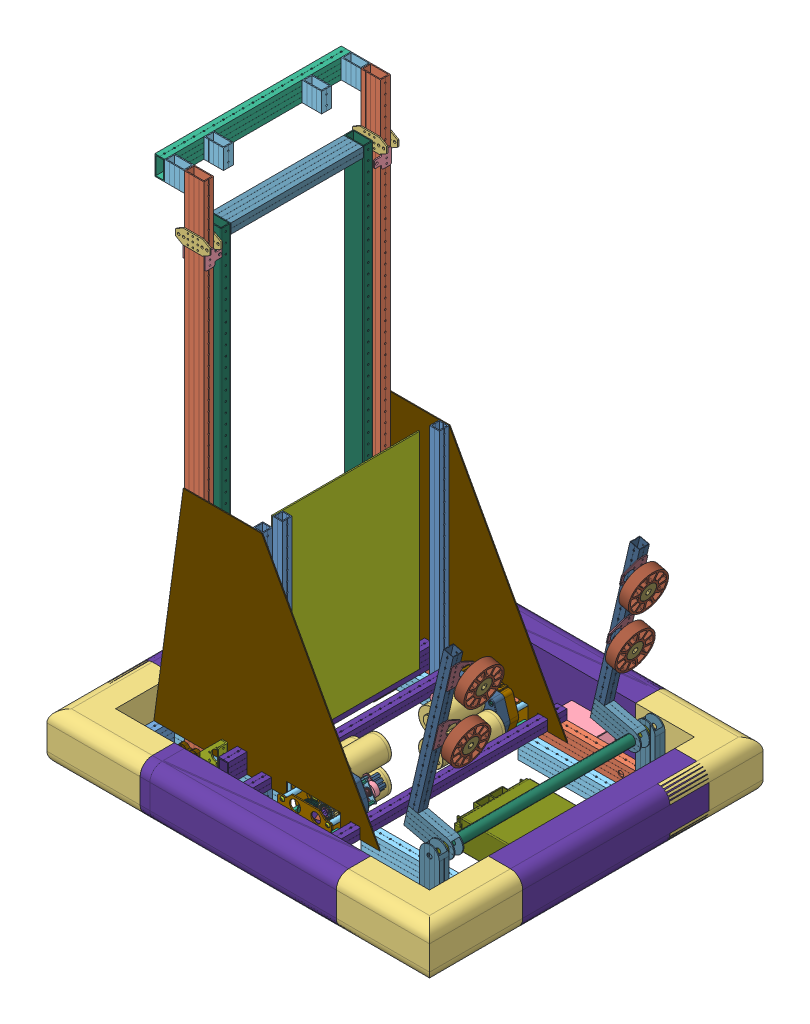
SolidWorks assembly FINAL BOT, configuration Default. Lengths in mm.
Overall size (1308.1 2133.6 883.55).
451 component instances, 126 part files, 82 mates.
Components (placement in the parent):
- Test Base 3-1: Test Base 3 [Default] at (-213.2986 -131.6714 217.4582) size (990.6 641.86 863.6)
  - Base Rear Rail-1: Base Rear Rail [Default] at (282.1219 360.9185 104.1623) size (25.4 50.8 685.8)
  - Base Side Rail-1: Base Side Rail [Default] at (1044.1219 360.9185 789.9623) x (0 0 1) z (-1 0 0) size (25.4 50.8 762)
  - Base Side Rail-2: Base Side Rail [Default] at (1044.1219 360.9185 231.1623) x (0 0 1) z (-1 0 0) size (25.4 50.8 762)
  - Blue Bumper-1: Blue Bumper [Default] at (1171.1219 335.5185 942.3623) x (0 0 -1) z (1 0 0) size (241.3 127 241.3)
  - Blue Bumper-2: Blue Bumper [Default] at (1171.1219 335.5185 78.7623) x (-1 0 0) z (0 0 -1) size (241.3 127 241.3)
  - Bumper Support Bar-2: Bumper Support Bar [Default] at (879.0219 335.5185 166.0294) x (0 0 1) z (-1 0 0) size (50.8 50.8 114.3)
  - Bumper Support Bar-4: Bumper Support Bar [Default] at (586.9219 335.5185 166.0294) x (0 0 1) z (-1 0 0) size (50.8 50.8 114.3)
  - Bumper Support Bar-7: Bumper Support Bar [Default] at (586.9219 335.5185 801.0294) x (0 0 1) z (-1 0 0) size (50.8 50.8 114.3)
  - Bumper Support Bar-8: Bumper Support Bar [Default] at (879.0219 335.5185 801.0294) x (0 0 1) z (-1 0 0) size (50.8 50.8 114.3)
  - Base Side Rail Internal-1: Base Side Rail Internal [Default] at (-175.0781 360.9185 713.7623) x (0 0 -1) z (1 0 0) size (25.4 50.8 279.4)
  - Base Side Rail Internal-4: Base Side Rail Internal [Default] at (1044.1219 360.9185 307.3623) x (0 0 1) z (-1 0 0) size (25.4 50.8 279.4)
  - Base Front Rail-1: Base Front Rail [Default] at (1069.5219 360.9185 104.1623) size (25.4 50.8 152.4)
  - 3 CIM Ball Shifter with WCD Output-1: 3 CIM Ball Shifter with WCD Output [Default] at (711.3612 400.7203 682.3171) x (0 1 0) z (0 0 1) size (169.11 183.68 312.65)
    - 217-2733-001 Rev2-1: 217-2733-001 Rev2 [Default] at (0 53.4162 37.6682) x (0 0 1) z (-0.00054 -1 0) size (7.11 24.61 24.61)
    - 217-2733-001 Rev2-2: 217-2733-001 Rev2 [Default] at (0 53.4162 7.9248) x (0 0 -1) z (-0.038475 0.99926 0) size (7.11 24.61 24.61)
    - 217-2731-001 Rev2-1: 217-2731-001 Rev2 [Default] at (0 0 0.0381) x (-0.099212 0.995066 0) z (0.995066 0.099212 0) size (31.12 7.94 31.12)
    - 217-2789-001 Rev2-1: 217-2789-001 Rev2 [Default] at (0 0 43.2943) x (0 0 -1) z (-0.58471 0.811243 0) size (11.1 38.4 38.4)
    - 217-2778-001 Rev2_NCQ8A075-050M_1-1: 217-2778-001 Rev2_NCQ8A075-050M_1 [Default] at (0 0 -53.848) x (-0.707107 0.707107 0) z (0 0 1) size (31.75 33.34 39.88)
      - 217-2778-002_075A-1: 217-2778-002_075A [Default] at origin size (31.75 33.34 26.92)
      - 217-2778-003_075M-1: 217-2778-003_075M [Default] at (0 0 -8.85) x (0.866025 -0.5 0) z (0 0 1) size (18.95 18.95 35.27)
      - 217-2778-004_075-1: 217-2778-004_075 [Default] at (0 0 10.362) size (21 20.74 0.97)
    - 217-2428-012 Rev2-1: 217-2428-012 Rev2 [Default] at (0 0 -40.386) size (63.5 22.23 2.29)
    - 217-2428-005 Rev1-1: 217-2428-005 Rev1 [Default] at (25.4 0 -19.05) x (-0.557362 -0.83027 0) z (-0.83027 0.557362 0) size (7.33 38.98 6.35)
    - 217-2428-005 Rev1-2: 217-2428-005 Rev1 [Default] at (-25.4 0 -19.05) x (0.667436 0.744667 0) z (0.744667 -0.667436 0) size (7.33 38.98 6.35)
    - SCREW-832-0375-1: SCREW-832-0375 [Default] at (25.4 0 -42.5958) x (0 0 1) z (-0.875404 0.483392 0) size (11.73 7.92 7.92)
    - SCREW-832-0375-2: SCREW-832-0375 [Default] at (-25.4 0 -42.5958) x (0 0 1) z (-0.966319 0.257347 0) size (11.73 7.92 7.92)
    - SCREW-832-0375-3: SCREW-832-0375 [Default] at (25.4 0 5.3848) x (0 0 -1) z (1 0 0) size (11.73 7.92 7.92)
    - SCREW-832-0375-4: SCREW-832-0375 [Default] at (-25.4 0 5.3848) x (0 0 -1) z (0.941463 -0.337115 0) size (11.73 7.92 7.92)
    - SBS1_SBS-0632-0250-1: SBS1_SBS-0632-0250 [Default] at (15.494 0 -36.2458) x (0 0 -1) z (0.854303 -0.519775 0) size (8.57 6.68 6.65)
    - SBS1_SBS-0632-0250-2: SBS1_SBS-0632-0250 [Default] at (-15.494 0 -36.2458) x (0 0 -1) z (0.854303 -0.519775 0) size (8.57 6.68 6.65)
    - 217-4098-100 Rev1-1: 217-4098-100 Rev1 [Default] at (0 0 -16.927) x (-0.503316 0.864103 0) z (0 0 1) size (18.03 19.79 22.46)
      - 217-4098-006 Rev2-1: 217-4098-006 Rev2 [Default] at (0 0 -4.6312) x (0 -1 0) z (0 0 -1) size (18.09 11.02 22.46)
      - 217-4098-006 Rev2-2: 217-4098-006 Rev2 [Default] at (0 0 -4.6312) x (0 1 0) z (0 0 -1) size (18.09 11.02 22.46)
      - 217-3489-001 Rev1-1: 217-3489-001 Rev1 [Default] at (0 0 -4.6312) x (0 0 1) z (-0.980217 -0.197926 0) size (4.77 12.7 12.7)
      - 97633A130_97633A130_grv-1: 97633A130_97633A130_grv [Default] at (0 0 -7.33) x (0 0 -1) z (0.979861 0.199683 0) size (0.64 8.74 7.34)
      - 91251A107_91251A107-1: 91251A107_91251A107 [Default] at (-4.8375 -6.735 -9.4343) x (0 0.863883 -0.503692) z (-1 0 0) size (4.65 4.65 10.79)
      - 91251A107_91251A107-2: 91251A107_91251A107 [Default] at (4.8375 6.735 -9.4343) x (0 0.470889 -0.882193) z (1 0 0) size (4.65 4.65 10.79)
    - 217-2428-017 Rev2-1: 217-2428-017 Rev2 [Default] at (12.7 -21.997 -3.614) x (-0.578458 -0.815712 0) z (0 0 -1) size (14.73 14.73 7.37)
    - 217-2428-016 Rev3_Spur01-1: 217-2428-016 Rev3_Spur01 [Default] at (0 0 -3.614) x (0.873157 -0.48744 0) z (0 0 1) size (40.67 40.74 13.32)
    - 217-2428-019 Rev1-1: 217-2428-019 Rev1 [Default] at (12.7 -21.997 -20.6248) x (0.866025 0.5 0) z (0 0 1) size (50.8 19.05 1.57)
    - 217-2428-006 Rev1-1: 217-2428-006 Rev1 [Default] at (32.079 -14.2875 -9.525) x (-0.752416 0.658689 0) z (0.658689 0.752416 0) size (7.33 19.93 6.35)
    - 217-2428-006 Rev1-2: 217-2428-006 Rev1 [Default] at (-3.6662 -34.925 -9.525) x (0.84498 0.534798 0) z (0.534798 -0.84498 0) size (7.33 19.93 6.35)
    - SCREW-832-0375-5: SCREW-832-0375 [Default] at (32.079 -14.2875 4.7498) x (0 0 -1) z (0.980613 0.195955 0) size (11.73 7.92 7.92)
    - SCREW-832-0375-6: SCREW-832-0375 [Default] at (-3.6662 -34.925 5.3848) x (0 0 -1) z (-0.672515 -0.740083 0) size (11.73 7.92 7.92)
    - SCREW-832-0375-7: SCREW-832-0375 [Default] at (-3.6662 -34.925 -22.8346) x (0 0 1) z (0.948865 0.315681 0) size (11.73 7.92 7.92)
    - SCREW-832-0375-8: SCREW-832-0375 [Default] at (32.079 -14.2875 -22.8346) x (0 0 1) z (-0.875404 0.483392 0) size (11.73 7.92 7.92)
    - 217-2614-001_12t-1: 217-2614-001_12t [Default] at (36.9798 39.6868 15.8623) x (-0.087156 0.996195 0) z (0 0 1) size (18.29 18.29 19)
    - 217-2761-001 rev1-1: 217-2761-001 rev1 [Default] at (33.1943 39.3556 16.1) x (0.087156 -0.996195 0) z (0 0 1) size (2 2 20)
    - 217-2761-001 rev1-2: 217-2761-001 rev1 [Default] at (-40.7653 40.018 16.1) x (0.087156 0.996195 0) z (0 0 1) size (2 2 20)
    - 217-2614-001_12t-2: 217-2614-001_12t [Default] at (-36.9798 39.6868 15.8623) x (0.087156 0.996195 0) z (0 0 1) size (18.29 18.29 19)
    - 217-2614-001_12t-3: 217-2614-001_12t [Default] at (0 92.8624 15.8623) x (0.97459 0.223996 0) z (0 0 1) size (18.29 18.29 19)
    - 217-2761-001 rev1-3: 217-2761-001 rev1 [Default] at (-0.8512 96.5658 16.1) x (0.97459 0.223996 0) z (0 0 1) size (2 2 20)
    - 217-3195-002 rev2-1: 217-3195-002 rev2 [Default] at (0 0 50.546) x (-1 0 0) z (0 0 -1) size (114.31 152.24 24.96)
    - 217-3195-001 Rev1-1: 217-3195-001 Rev1 [Default] at origin size (113.41 152.24 26.86)
    - Nylock Nut_NNY2520-ZC-1: Nylock Nut_NNY2520-ZC [Default] at (48.8823 73.025 37.846) x (0 0.866025 -0.5) z (-1 0 0) size (12.85 11.89 7.62)
    - Nylock Nut_NNY2520-ZC-2: Nylock Nut_NNY2520-ZC [Default] at (48.8823 -3.175 37.846) x (0 0 -1) z (-1 0 0) size (12.85 11.89 7.62)
    - Nylock Nut_NNY2520-ZC-3: Nylock Nut_NNY2520-ZC [Default] at (44.45 85.725 7.8613) x (0 1 0) z (0 0 -1) size (12.85 11.89 7.62)
    - 276-1027-001-1: 276-1027-001 [Default] at (47.625 58.1787 6.35) x (0 1 0) z (-1 0 0) size (8.61 5.64 9.94)
    - 276-1027-001-2: 276-1027-001 [Default] at (-47.625 58.1787 6.35) x (0 -1 0) z (1 0 0) size (8.61 5.64 9.94)
    - SCREW-832-1750-1: SCREW-832-1750 [Default] at (-47.625 58.1787 47.0408) x (0 0 -1) z (-0.960822 -0.277167 0) size (46.66 7.92 7.92)
    - SCREW-832-1750-2: SCREW-832-1750 [Default] at (47.625 58.1787 47.0408) x (0 0 -1) z (-0.960822 -0.277167 0) size (46.66 7.92 7.92)
    - Nylock Nut_NNY2520-ZC-4: Nylock Nut_NNY2520-ZC [Default] at (44.45 -15.875 7.8613) x (0 1 0) z (0 0 -1) size (12.85 11.89 7.62)
    - 217-2428-004 Rev3-1: 217-2428-004 Rev3 [Default] at (0 53.4162 22.7711) x (-0.709585 0.70462 0) z (0 0 1) size (11 9.53 43.92)
    - SBS1_SBS-2520-1625SS-1: SBS1_SBS-2520-1625SS [Default] at (44.45 85.725 42.4688) x (0 0 -1) z (-0.251219 0.96793 0) size (45.3 11.2 11.18)
    - SBS1_SBS-2520-1625SS-2: SBS1_SBS-2520-1625SS [Default] at (44.45 -15.875 42.4688) x (0 0 -1) z (-0.251219 0.96793 0) size (45.3 11.2 11.18)
    - SBS1_SBS2520-1750-1: SBS1_SBS2520-1750 [Default] at (-44.45 85.725 7.4422) x (0 0 1) z (-0.031478 0.999504 0) size (48.48 11.22 11.17)
    - SBS1_SBS2520-1750-2: SBS1_SBS2520-1750 [Default] at (-44.45 -15.875 7.4422) x (0 0 1) z (-0.937114 -0.349025 0) size (48.48 11.22 11.17)
    - 217-2428-021 Rev1-1: 217-2428-021 Rev1 [Default] at (0 53.4162 9.5123) x (0.451333 -0.892356 0) z (0 0 1) size (15.88 15.88 3.17)
    - 217-2428-029 Rev1-1: 217-2428-029 Rev1 [Default] at (0 53.4162 36.957) x (0.999846 0.017557 0) z (0 0 1) size (15.88 15.88 1.12)
    - Grayhill Lock Washer-1: Grayhill Lock Washer [Default] at (12.7 -21.997 -18.6817) x (0.467173 -0.884166 0) z (0 0 1) size (19.69 19.69 0.74)
    - Grayhill Nut-1: Grayhill Nut [Default] at (12.7 -21.997 -17.0434) x (0.984088 0.177684 0) z (0 0 1) size (18.33 15.88 2.54)
    - 217-2000-1: 217-2000 [Default] at (0 92.8624 0) x (0 0 -1) z (0.223996 -0.97459 0) size (150.2 64.01 64.01)
    - 217-2000-2: 217-2000 [Default] at (-36.9798 39.6868 0) x (0 0 -1) z (0.996195 -0.087156 0) size (150.2 64.01 64.01)
    - 217-2000-3: 217-2000 [Default] at (36.9798 39.6868 0) x (0 0 -1) z (0.996195 0.087156 0) size (150.2 64.01 64.01)
    - Grahill Encoder-1: Grahill Encoder [Default] at (12.7 -21.997 -16.1798) x (-0.580071 0.814566 0) z (-0.814566 -0.580071 0) size (31.75 31.12 31.75)
    - 217-3195-009 Rev1_wcd 2-1: 217-3195-009 Rev1_wcd 2 [Default] at (0 85.725 50.546) x (-0.998427 -0.056065 0) z (0 0 1) size (12.7 12.7 41.27)
    - 217-3195-006 Rev1_WCD-1: 217-3195-006 Rev1_WCD [Default] at (-44.45 85.725 44.1452) x (0.5 0.866025 0) z (0 0 1) size (12.7 14.66 47.62)
    - 217-3195-009 Rev1_wcd 2-2: 217-3195-009 Rev1_wcd 2 [Default] at (0 -31.75 50.546) x (0.947633 0.319361 0) z (0 0 1) size (12.7 12.7 41.27)
    - 217-3195-006 Rev1_WCD-2: 217-3195-006 Rev1_WCD [Default] at (-44.45 -15.875 44.1452) x (0.5 -0.866025 0) z (0 0 1) size (12.7 14.66 47.62)
    - Nylock Nut_NNY2520-ZC-5: Nylock Nut_NNY2520-ZC [Default] at (0 -31.75 45.0723) x (-0.5 0.866025 0) z (0 0 -1) size (12.85 11.89 7.62)
    - Nylock Nut_NNY2520-ZC-6: Nylock Nut_NNY2520-ZC [Default] at (0 85.725 45.0723) x (-0.5 0.866025 0) z (0 0 -1) size (12.85 11.89 7.62)
    - SBS1_SBS-2520-2250-1: SBS1_SBS-2520-2250 [Default] at (0 -31.75 98.298) x (0 0 -1) z (-0.933488 -0.358607 0) size (61.18 11.22 11.17)
    - SBS1_SBS2520-0625ZC-1: SBS1_SBS2520-0625ZC [Default] at (-44.45 85.725 98.298) x (0 0 -1) z (0.400817 0.916158 0) size (19.57 11.22 11.17)
    - SBS1_SBS2520-0625ZC-2: SBS1_SBS2520-0625ZC [Default] at (-44.45 -15.875 98.298) x (0 0 -1) z (-0.75178 -0.659414 0) size (19.57 11.22 11.17)
    - SBS1_SBS-2520-2250-2: SBS1_SBS-2520-2250 [Default] at (0 85.725 98.298) x (0 0 -1) z (0.056677 -0.998393 0) size (61.18 11.22 11.17)
    - 217-3195-003 rev2-1: 217-3195-003 rev2 [Default] at (0 0 94.9452) size (88.62 139.7 3.17)
    - 217-2617-003 Rev1-1: 217-2617-003 Rev1 [Default] at (-39.878 35.5392 121.8535) x (-0.5 -0.866025 0) z (0 0 1) size (14.66 12.7 152.4)
    - 217-3109-001 Rev1-1: 217-3109-001 Rev1 [Default] at (-39.878 35.5392 49.1808) x (0 0 1) z (0.312889 -0.94979 0) size (7.94 28.57 28.57)
    - 217-2734-001 Rev3-1: 217-2734-001 Rev3 [Default] at (-39.878 35.5392 98.1202) x (1 0 0) z (0 1 0) size (31.12 7.94 31.12)
    - 217-2617-004 Rev1_97431A340_grv-1: 217-2617-004 Rev1_97431A340_grv [Default] at (-39.878 35.5392 54.8961) x (0 0 1) z (-0.124043 -0.992277 0) size (1.07 20.42 18.58)
    - 217-2617-004 Rev1_97431A340_grv-2: 217-2617-004 Rev1_97431A340_grv [Default] at (0 0 69.215) x (0 0 1) z (-0.124043 -0.992277 0) size (1.07 20.42 18.58)
    - 217-2702-001_20t-1: 217-2702-001_20t [Default] at (0 0 62.357) x (0.998435 0.055929 0) z (0 0 1) size (28.2 28.2 12.65)
    - 217-2715-002 Rev1_64t-1: 217-2715-002 Rev1_64t [Default] at (-39.878 35.5392 61.7541) x (0.866025 -0.5 0) z (0 0 1) size (84.3 84.3 12.65)
    - 217-2704-001_24-1: 217-2704-001_24 [Default] at (0 0 62.357) x (0.450781 0.892635 0) z (0 0 -1) size (33.29 33.29 12.65)
    - 217-2714-002 Rev1_60t-1: 217-2714-002 Rev1_60t [Default] at (-39.878 35.5392 61.7541) x (0.866025 -0.5 0) z (0 0 1) size (78.95 78.95 12.65)
    - 217-3221-002 Rev1-1: 217-3221-002 Rev1 [Default] at (-39.878 35.5392 61.7414) x (0 -1 0) z (0 0 1) size (71.39 71.45 12.62)
    - 217-2705-001_30t-1: 217-2705-001_30t [Default] at (0 0 62.357) x (0.547654 -0.836705 0) z (0 0 1) size (41.01 41.12 12.65)
    - 217-2712-002 Rev1_50t-1: 217-2712-002 Rev1_50t [Default] at (-39.878 35.5392 61.7541) x (0.866025 -0.5 0) z (0 0 1) size (66.7 66.76 12.65)
    - 217-2706-001_34t-1: 217-2706-001_34t [Default] at (0 0 62.357) x (0.998435 0.055929 0) z (0 0 1) size (46.46 46.56 12.65)
    - 217-3288-001 Rev3-1: 217-3288-001 Rev3 [Default] at (0 0 0.0889) x (0.055929 -0.998435 0) z (0 0 1) size (99.51 99.53 98.3)
      - 217-2428-008 Rev2-1: 217-2428-008 Rev2 [Default] at (0 0 10.2679) size (31.75 31.75 1.59)
      - 217-2428-028 Rev1_97633A250-1: 217-2428-028 Rev1_97633A250 [Default] at (0 0 37.1221) x (0 0 1) z (0.9357 -0.352797 0) size (1.07 23.39 21.18)
      - 217-4099-000 Rev2_high gear-1: 217-4099-000 Rev2_high gear [Default] x (-1 0 0) z (0 0 1) size (22.23 22.23 98.3)
        - 217-4098-005 Rev1_91612A226-1: 217-4098-005 Rev1_91612A226 [Default] at (0 0 46.2661) x (-0.144757 0 0.989467) z (0 -1 0) size (3.02 3.15 18.22)
        - 217-4098-003 Rev2-1: 217-4098-003 Rev2 [Default] x (1 0 0) z (0 0 -1) size (22.23 22.23 55.94)
        - 217-4099-002 Rev3-1: 217-4099-002 Rev3 [Default] at (0 0 53.467) x (0 0 1) z (-1 0 0) size (40.96 12.73 14.67)
        - 217-4098-004 Rev1-1: 217-4098-004 Rev1 [Default] at (0 0 14.2494) x (0.393904 0.919152 0) z (0 0 1) size (11.68 11.68 56)
      - 217-2428-007 Rev1-1: 217-2428-007 Rev1 [Default] at (7.809 4.5085 14.2494) x (-0.69071 0.455693 -0.561483) z (-0.67559 -0.683536 0.276329) size (6.35 6.35 6.35)
      - 217-2428-007 Rev1-2: 217-2428-007 Rev1 [Default] at (5.4343 3.1375 26.9494) x (-0.162331 -0.978398 0.128005) z (0.857281 -0.204076 -0.472676) size (6.35 6.35 6.35)
      - 217-3212-101 Rev1-1: 217-3212-101 Rev1 [Default] at (-11.5751 10.4131 45.3224) x (0.923728 0.383049 0) z (0 0 -1) size (46.46 46.56 12.7)
        - 217-2428-022 Rev1-1: 217-2428-022 Rev1 [Default] at (6.7035 14.0527 24.6087) size (28.57 28.57 6.1)
        - 217-3212-001 Rev1_34t-1: 217-3212-001 Rev1_34t [Default] at (6.7035 14.0527 27.9107) size (46.46 46.56 11.11)
      - 217-3222-101 Rev1-1: 217-3222-101 Rev1 [Default] at (21.0941 -5.2804 52.7371) x (-0.889163 -0.457591 0) z (0 0 -1) size (73.87 73.92 12.7)
        - 217-2428-022 Rev1-1: 217-2428-022 Rev1 [Default] at (16.3398 14.3476 19.3234) size (28.57 28.57 6.1)
        - 217-3222-001 Rev1_Spur01-1: 217-3222-001 Rev1_Spur01 [Default] at (16.3398 14.3476 22.6254) x (0.999377 0.0353 0) z (0 0 1) size (71.39 71.45 11.11)
      - 217-2428-007 Rev1-3: 217-2428-007 Rev1 [Default] at (-5.4343 3.1375 26.9494) x (0.928483 0.348617 0.128005) z (-0.251905 0.844465 -0.472676) size (6.35 6.35 6.35)
      - 217-2428-007 Rev1-4: 217-2428-007 Rev1 [Default] at (0 -6.275 26.9494) x (-0.766153 0.629782 0.128005) z (-0.605376 -0.640389 -0.472676) size (6.35 6.35 6.35)
      - 217-2428-007 Rev1-5: 217-2428-007 Rev1 [Default] at (-7.809 4.5085 14.2494) x (-0.049287 -0.826019 -0.561483) z (0.929754 -0.24331 0.276329) size (6.35 6.35 6.35)
      - 217-2428-007 Rev1-6: 217-2428-007 Rev1 [Default] at (0 -9.017 14.2494) x (0.739997 0.370326 -0.561483) z (-0.254164 0.926846 0.276329) size (6.35 6.35 6.35)
    - 217-3210-001 Rev1_30t-1: 217-3210-001 Rev1_30t [Default] at (0 53.4162 30.0736) x (-0.966828 0.255427 0) z (0 0 1) size (41.01 41.12 12.65)
    - 217-2711-002 Rev1_50t-1: 217-2711-002 Rev1_50t [Default] at (0 53.4162 17.4244) x (0.262208 -0.965011 0) z (0 0 1) size (66.7 66.76 12.65)
  - 3 CIM Ball Shifter with WCD Output-2: 3 CIM Ball Shifter with WCD Output [Default] at (640.2827 400.7203 338.8075) x (0 1 0) z (0 0 -1) size (169.11 183.68 312.65)
    - 217-2733-001 Rev2-1: 217-2733-001 Rev2 [Default] at (0 53.4162 37.6682) x (0 0 1) z (-0.00054 -1 0) size (7.11 24.61 24.61)
    - 217-2733-001 Rev2-2: 217-2733-001 Rev2 [Default] at (0 53.4162 7.9248) x (0 0 -1) z (-0.038475 0.99926 0) size (7.11 24.61 24.61)
    - 217-2731-001 Rev2-1: 217-2731-001 Rev2 [Default] at (0 0 0.0381) x (-0.099212 0.995066 0) z (0.995066 0.099212 0) size (31.12 7.94 31.12)
    - 217-2789-001 Rev2-1: 217-2789-001 Rev2 [Default] at (0 0 43.2943) x (0 0 -1) z (-0.58471 0.811243 0) size (11.1 38.4 38.4)
    - 217-2778-001 Rev2_NCQ8A075-050M_1-1: 217-2778-001 Rev2_NCQ8A075-050M_1 [Default] at (0 0 -53.848) x (-0.707107 0.707107 0) z (0 0 1) size (31.75 33.34 39.88)
      - 217-2778-002_075A-1: 217-2778-002_075A [Default] at origin size (31.75 33.34 26.92)
      - 217-2778-003_075M-1: 217-2778-003_075M [Default] at (0 0 -8.85) x (0.866025 -0.5 0) z (0 0 1) size (18.95 18.95 35.27)
      - 217-2778-004_075-1: 217-2778-004_075 [Default] at (0 0 10.362) size (21 20.74 0.97)
    - 217-2428-012 Rev2-1: 217-2428-012 Rev2 [Default] at (0 0 -40.386) size (63.5 22.23 2.29)
    - 217-2428-005 Rev1-1: 217-2428-005 Rev1 [Default] at (25.4 0 -19.05) x (-0.557362 -0.83027 0) z (-0.83027 0.557362 0) size (7.33 38.98 6.35)
    - 217-2428-005 Rev1-2: 217-2428-005 Rev1 [Default] at (-25.4 0 -19.05) x (0.667436 0.744667 0) z (0.744667 -0.667436 0) size (7.33 38.98 6.35)
    - SCREW-832-0375-1: SCREW-832-0375 [Default] at (25.4 0 -42.5958) x (0 0 1) z (-0.875404 0.483392 0) size (11.73 7.92 7.92)
    - SCREW-832-0375-2: SCREW-832-0375 [Default] at (-25.4 0 -42.5958) x (0 0 1) z (-0.966319 0.257347 0) size (11.73 7.92 7.92)
    - SCREW-832-0375-3: SCREW-832-0375 [Default] at (25.4 0 5.3848) x (0 0 -1) z (1 0 0) size (11.73 7.92 7.92)
    - SCREW-832-0375-4: SCREW-832-0375 [Default] at (-25.4 0 5.3848) x (0 0 -1) z (0.941463 -0.337115 0) size (11.73 7.92 7.92)
    - SBS1_SBS-0632-0250-1: SBS1_SBS-0632-0250 [Default] at (15.494 0 -36.2458) x (0 0 -1) z (0.854303 -0.519775 0) size (8.57 6.68 6.65)
    - SBS1_SBS-0632-0250-2: SBS1_SBS-0632-0250 [Default] at (-15.494 0 -36.2458) x (0 0 -1) z (0.854303 -0.519775 0) size (8.57 6.68 6.65)
    - 217-4098-100 Rev1-1: 217-4098-100 Rev1 [Default] at (0 0 -16.927) x (-0.503316 0.864103 0) z (0 0 1) size (18.03 19.79 22.46)
      - 217-4098-006 Rev2-1: 217-4098-006 Rev2 [Default] at (0 0 -4.6312) x (0 -1 0) z (0 0 -1) size (18.09 11.02 22.46)
      - 217-4098-006 Rev2-2: 217-4098-006 Rev2 [Default] at (0 0 -4.6312) x (0 1 0) z (0 0 -1) size (18.09 11.02 22.46)
      - 217-3489-001 Rev1-1: 217-3489-001 Rev1 [Default] at (0 0 -4.6312) x (0 0 1) z (-0.980217 -0.197926 0) size (4.77 12.7 12.7)
      - 97633A130_97633A130_grv-1: 97633A130_97633A130_grv [Default] at (0 0 -7.33) x (0 0 -1) z (0.979861 0.199683 0) size (0.64 8.74 7.34)
      - 91251A107_91251A107-1: 91251A107_91251A107 [Default] at (-4.8375 -6.735 -9.4343) x (0 0.863883 -0.503692) z (-1 0 0) size (4.65 4.65 10.79)
      - 91251A107_91251A107-2: 91251A107_91251A107 [Default] at (4.8375 6.735 -9.4343) x (0 0.470889 -0.882193) z (1 0 0) size (4.65 4.65 10.79)
    - 217-2428-017 Rev2-1: 217-2428-017 Rev2 [Default] at (12.7 -21.997 -3.614) x (-0.578458 -0.815712 0) z (0 0 -1) size (14.73 14.73 7.37)
    - 217-2428-016 Rev3_Spur01-1: 217-2428-016 Rev3_Spur01 [Default] at (0 0 -3.614) x (0.873157 -0.48744 0) z (0 0 1) size (40.67 40.74 13.32)
    - 217-2428-019 Rev1-1: 217-2428-019 Rev1 [Default] at (12.7 -21.997 -20.6248) x (0.866025 0.5 0) z (0 0 1) size (50.8 19.05 1.57)
    - 217-2428-006 Rev1-1: 217-2428-006 Rev1 [Default] at (32.079 -14.2875 -9.525) x (-0.752416 0.658689 0) z (0.658689 0.752416 0) size (7.33 19.93 6.35)
    - 217-2428-006 Rev1-2: 217-2428-006 Rev1 [Default] at (-3.6662 -34.925 -9.525) x (0.84498 0.534798 0) z (0.534798 -0.84498 0) size (7.33 19.93 6.35)
    - SCREW-832-0375-5: SCREW-832-0375 [Default] at (32.079 -14.2875 4.7498) x (0 0 -1) z (0.980613 0.195955 0) size (11.73 7.92 7.92)
    - SCREW-832-0375-6: SCREW-832-0375 [Default] at (-3.6662 -34.925 5.3848) x (0 0 -1) z (-0.672515 -0.740083 0) size (11.73 7.92 7.92)
    - SCREW-832-0375-7: SCREW-832-0375 [Default] at (-3.6662 -34.925 -22.8346) x (0 0 1) z (0.948865 0.315681 0) size (11.73 7.92 7.92)
    - SCREW-832-0375-8: SCREW-832-0375 [Default] at (32.079 -14.2875 -22.8346) x (0 0 1) z (-0.875404 0.483392 0) size (11.73 7.92 7.92)
    - 217-2614-001_12t-1: 217-2614-001_12t [Default] at (36.9798 39.6868 15.8623) x (-0.087156 0.996195 0) z (0 0 1) size (18.29 18.29 19)
    - 217-2761-001 rev1-1: 217-2761-001 rev1 [Default] at (33.1943 39.3556 16.1) x (0.087156 -0.996195 0) z (0 0 1) size (2 2 20)
    - 217-2761-001 rev1-2: 217-2761-001 rev1 [Default] at (-40.7653 40.018 16.1) x (0.087156 0.996195 0) z (0 0 1) size (2 2 20)
    - 217-2614-001_12t-2: 217-2614-001_12t [Default] at (-36.9798 39.6868 15.8623) x (0.087156 0.996195 0) z (0 0 1) size (18.29 18.29 19)
    - 217-2614-001_12t-3: 217-2614-001_12t [Default] at (0 92.8624 15.8623) x (0.97459 0.223996 0) z (0 0 1) size (18.29 18.29 19)
    - 217-2761-001 rev1-3: 217-2761-001 rev1 [Default] at (-0.8512 96.5658 16.1) x (0.97459 0.223996 0) z (0 0 1) size (2 2 20)
    - 217-3195-002 rev2-1: 217-3195-002 rev2 [Default] at (0 0 50.546) x (-1 0 0) z (0 0 -1) size (114.31 152.24 24.96)
    - 217-3195-001 Rev1-1: 217-3195-001 Rev1 [Default] at origin size (113.41 152.24 26.86)
    - Nylock Nut_NNY2520-ZC-1: Nylock Nut_NNY2520-ZC [Default] at (48.8823 73.025 37.846) x (0 0.866025 -0.5) z (-1 0 0) size (12.85 11.89 7.62)
    - Nylock Nut_NNY2520-ZC-2: Nylock Nut_NNY2520-ZC [Default] at (48.8823 -3.175 37.846) x (0 0 -1) z (-1 0 0) size (12.85 11.89 7.62)
    - Nylock Nut_NNY2520-ZC-3: Nylock Nut_NNY2520-ZC [Default] at (44.45 85.725 7.8613) x (0 1 0) z (0 0 -1) size (12.85 11.89 7.62)
    - 276-1027-001-1: 276-1027-001 [Default] at (47.625 58.1787 6.35) x (0 1 0) z (-1 0 0) size (8.61 5.64 9.94)
    - 276-1027-001-2: 276-1027-001 [Default] at (-47.625 58.1787 6.35) x (0 -1 0) z (1 0 0) size (8.61 5.64 9.94)
    - SCREW-832-1750-1: SCREW-832-1750 [Default] at (-47.625 58.1787 47.0408) x (0 0 -1) z (-0.960822 -0.277167 0) size (46.66 7.92 7.92)
    - SCREW-832-1750-2: SCREW-832-1750 [Default] at (47.625 58.1787 47.0408) x (0 0 -1) z (-0.960822 -0.277167 0) size (46.66 7.92 7.92)
    - Nylock Nut_NNY2520-ZC-4: Nylock Nut_NNY2520-ZC [Default] at (44.45 -15.875 7.8613) x (0 1 0) z (0 0 -1) size (12.85 11.89 7.62)
    - 217-2428-004 Rev3-1: 217-2428-004 Rev3 [Default] at (0 53.4162 22.7711) x (-0.709585 0.70462 0) z (0 0 1) size (11 9.53 43.92)
    - SBS1_SBS-2520-1625SS-1: SBS1_SBS-2520-1625SS [Default] at (44.45 85.725 42.4688) x (0 0 -1) z (-0.251219 0.96793 0) size (45.3 11.2 11.18)
    - SBS1_SBS-2520-1625SS-2: SBS1_SBS-2520-1625SS [Default] at (44.45 -15.875 42.4688) x (0 0 -1) z (-0.251219 0.96793 0) size (45.3 11.2 11.18)
    - SBS1_SBS2520-1750-1: SBS1_SBS2520-1750 [Default] at (-44.45 85.725 7.4422) x (0 0 1) z (-0.031478 0.999504 0) size (48.48 11.22 11.17)
    - SBS1_SBS2520-1750-2: SBS1_SBS2520-1750 [Default] at (-44.45 -15.875 7.4422) x (0 0 1) z (-0.937114 -0.349025 0) size (48.48 11.22 11.17)
    - 217-2428-021 Rev1-1: 217-2428-021 Rev1 [Default] at (0 53.4162 9.5123) x (0.451333 -0.892356 0) z (0 0 1) size (15.88 15.88 3.17)
    - 217-2428-029 Rev1-1: 217-2428-029 Rev1 [Default] at (0 53.4162 36.957) x (0.999846 0.017557 0) z (0 0 1) size (15.88 15.88 1.12)
    - Grayhill Lock Washer-1: Grayhill Lock Washer [Default] at (12.7 -21.997 -18.6817) x (0.467173 -0.884166 0) z (0 0 1) size (19.69 19.69 0.74)
    - Grayhill Nut-1: Grayhill Nut [Default] at (12.7 -21.997 -17.0434) x (0.984088 0.177684 0) z (0 0 1) size (18.33 15.88 2.54)
    - 217-2000-1: 217-2000 [Default] at (0 92.8624 0) x (0 0 -1) z (0.223996 -0.97459 0) size (150.2 64.01 64.01)
    - 217-2000-2: 217-2000 [Default] at (-36.9798 39.6868 0) x (0 0 -1) z (0.996195 -0.087156 0) size (150.2 64.01 64.01)
    - 217-2000-3: 217-2000 [Default] at (36.9798 39.6868 0) x (0 0 -1) z (0.996195 0.087156 0) size (150.2 64.01 64.01)
    - Grahill Encoder-1: Grahill Encoder [Default] at (12.7 -21.997 -16.1798) x (-0.580071 0.814566 0) z (-0.814566 -0.580071 0) size (31.75 31.12 31.75)
    - 217-3195-009 Rev1_wcd 2-1: 217-3195-009 Rev1_wcd 2 [Default] at (0 85.725 50.546) x (-0.998427 -0.056065 0) z (0 0 1) size (12.7 12.7 41.27)
    - 217-3195-006 Rev1_WCD-1: 217-3195-006 Rev1_WCD [Default] at (-44.45 85.725 44.1452) x (0.5 0.866025 0) z (0 0 1) size (12.7 14.66 47.62)
    - 217-3195-009 Rev1_wcd 2-2: 217-3195-009 Rev1_wcd 2 [Default] at (0 -31.75 50.546) x (0.947633 0.319361 0) z (0 0 1) size (12.7 12.7 41.27)
    - 217-3195-006 Rev1_WCD-2: 217-3195-006 Rev1_WCD [Default] at (-44.45 -15.875 44.1452) x (0.5 -0.866025 0) z (0 0 1) size (12.7 14.66 47.62)
    - Nylock Nut_NNY2520-ZC-5: Nylock Nut_NNY2520-ZC [Default] at (0 -31.75 45.0723) x (-0.5 0.866025 0) z (0 0 -1) size (12.85 11.89 7.62)
    - Nylock Nut_NNY2520-ZC-6: Nylock Nut_NNY2520-ZC [Default] at (0 85.725 45.0723) x (-0.5 0.866025 0) z (0 0 -1) size (12.85 11.89 7.62)
    - SBS1_SBS-2520-2250-1: SBS1_SBS-2520-2250 [Default] at (0 -31.75 98.298) x (0 0 -1) z (-0.933488 -0.358607 0) size (61.18 11.22 11.17)
    - SBS1_SBS2520-0625ZC-1: SBS1_SBS2520-0625ZC [Default] at (-44.45 85.725 98.298) x (0 0 -1) z (0.400817 0.916158 0) size (19.57 11.22 11.17)
    - SBS1_SBS2520-0625ZC-2: SBS1_SBS2520-0625ZC [Default] at (-44.45 -15.875 98.298) x (0 0 -1) z (-0.75178 -0.659414 0) size (19.57 11.22 11.17)
    - SBS1_SBS-2520-2250-2: SBS1_SBS-2520-2250 [Default] at (0 85.725 98.298) x (0 0 -1) z (0.056677 -0.998393 0) size (61.18 11.22 11.17)
    - 217-3195-003 rev2-1: 217-3195-003 rev2 [Default] at (0 0 94.9452) size (88.62 139.7 3.17)
    - 217-2617-003 Rev1-1: 217-2617-003 Rev1 [Default] at (-39.878 35.5392 121.8535) x (-0.5 -0.866025 0) z (0 0 1) size (14.66 12.7 152.4)
    - 217-3109-001 Rev1-1: 217-3109-001 Rev1 [Default] at (-39.878 35.5392 49.1808) x (0 0 1) z (0.312889 -0.94979 0) size (7.94 28.57 28.57)
    - 217-2734-001 Rev3-1: 217-2734-001 Rev3 [Default] at (-39.878 35.5392 98.1202) x (1 0 0) z (0 1 0) size (31.12 7.94 31.12)
    - 217-2617-004 Rev1_97431A340_grv-1: 217-2617-004 Rev1_97431A340_grv [Default] at (-39.878 35.5392 54.8961) x (0 0 1) z (-0.124043 -0.992277 0) size (1.07 20.42 18.58)
    - 217-2617-004 Rev1_97431A340_grv-2: 217-2617-004 Rev1_97431A340_grv [Default] at (0 0 69.215) x (0 0 1) z (-0.124043 -0.992277 0) size (1.07 20.42 18.58)
    - 217-2702-001_20t-1: 217-2702-001_20t [Default] at (0 0 62.357) x (0.998435 0.055929 0) z (0 0 1) size (28.2 28.2 12.65)
    - 217-2715-002 Rev1_64t-1: 217-2715-002 Rev1_64t [Default] at (-39.878 35.5392 61.7541) x (0.866025 -0.5 0) z (0 0 1) size (84.3 84.3 12.65)
    - 217-2704-001_24-1: 217-2704-001_24 [Default] at (0 0 62.357) x (0.450781 0.892635 0) z (0 0 -1) size (33.29 33.29 12.65)
    - 217-2714-002 Rev1_60t-1: 217-2714-002 Rev1_60t [Default] at (-39.878 35.5392 61.7541) x (0.866025 -0.5 0) z (0 0 1) size (78.95 78.95 12.65)
    - 217-3221-002 Rev1-1: 217-3221-002 Rev1 [Default] at (-39.878 35.5392 61.7414) x (0 -1 0) z (0 0 1) size (71.39 71.45 12.62)
    - 217-2705-001_30t-1: 217-2705-001_30t [Default] at (0 0 62.357) x (0.547654 -0.836705 0) z (0 0 1) size (41.01 41.12 12.65)
    - 217-2712-002 Rev1_50t-1: 217-2712-002 Rev1_50t [Default] at (-39.878 35.5392 61.7541) x (0.866025 -0.5 0) z (0 0 1) size (66.7 66.76 12.65)
    - 217-2706-001_34t-1: 217-2706-001_34t [Default] at (0 0 62.357) x (0.998435 0.055929 0) z (0 0 1) size (46.46 46.56 12.65)
    - 217-3288-001 Rev3-1: 217-3288-001 Rev3 [Default] at (0 0 0.0889) x (0.055929 -0.998435 0) z (0 0 1) size (99.51 99.53 98.3)
      - 217-2428-008 Rev2-1: 217-2428-008 Rev2 [Default] at (0 0 10.2679) size (31.75 31.75 1.59)
      - 217-2428-028 Rev1_97633A250-1: 217-2428-028 Rev1_97633A250 [Default] at (0 0 37.1221) x (0 0 1) z (0.9357 -0.352797 0) size (1.07 23.39 21.18)
      - 217-4099-000 Rev2_high gear-1: 217-4099-000 Rev2_high gear [Default] x (-1 0 0) z (0 0 1) size (22.23 22.23 98.3)
        - 217-4098-005 Rev1_91612A226-1: 217-4098-005 Rev1_91612A226 [Default] at (0 0 46.2661) x (-0.144757 0 0.989467) z (0 -1 0) size (3.02 3.15 18.22)
        - 217-4098-003 Rev2-1: 217-4098-003 Rev2 [Default] x (1 0 0) z (0 0 -1) size (22.23 22.23 55.94)
        - 217-4099-002 Rev3-1: 217-4099-002 Rev3 [Default] at (0 0 53.467) x (0 0 1) z (-1 0 0) size (40.96 12.73 14.67)
        - 217-4098-004 Rev1-1: 217-4098-004 Rev1 [Default] at (0 0 14.2494) x (0.393904 0.919152 0) z (0 0 1) size (11.68 11.68 56)
      - 217-2428-007 Rev1-1: 217-2428-007 Rev1 [Default] at (7.809 4.5085 14.2494) x (-0.69071 0.455693 -0.561483) z (-0.67559 -0.683536 0.276329) size (6.35 6.35 6.35)
      - 217-2428-007 Rev1-2: 217-2428-007 Rev1 [Default] at (5.4343 3.1375 26.9494) x (-0.162331 -0.978398 0.128005) z (0.857281 -0.204076 -0.472676) size (6.35 6.35 6.35)
      - 217-3212-101 Rev1-1: 217-3212-101 Rev1 [Default] at (-11.5751 10.4131 45.3224) x (0.923728 0.383049 0) z (0 0 -1) size (46.46 46.56 12.7)
        - 217-2428-022 Rev1-1: 217-2428-022 Rev1 [Default] at (6.7035 14.0527 24.6087) size (28.57 28.57 6.1)
        - 217-3212-001 Rev1_34t-1: 217-3212-001 Rev1_34t [Default] at (6.7035 14.0527 27.9107) size (46.46 46.56 11.11)
      - 217-3222-101 Rev1-1: 217-3222-101 Rev1 [Default] at (21.0941 -5.2804 52.7371) x (-0.889163 -0.457591 0) z (0 0 -1) size (73.87 73.92 12.7)
        - 217-2428-022 Rev1-1: 217-2428-022 Rev1 [Default] at (16.3398 14.3476 19.3234) size (28.57 28.57 6.1)
        - 217-3222-001 Rev1_Spur01-1: 217-3222-001 Rev1_Spur01 [Default] at (16.3398 14.3476 22.6254) x (0.999377 0.0353 0) z (0 0 1) size (71.39 71.45 11.11)
      - 217-2428-007 Rev1-3: 217-2428-007 Rev1 [Default] at (-5.4343 3.1375 26.9494) x (0.928483 0.348617 0.128005) z (-0.251905 0.844465 -0.472676) size (6.35 6.35 6.35)
      - 217-2428-007 Rev1-4: 217-2428-007 Rev1 [Default] at (0 -6.275 26.9494) x (-0.766153 0.629782 0.128005) z (-0.605376 -0.640389 -0.472676) size (6.35 6.35 6.35)
      - 217-2428-007 Rev1-5: 217-2428-007 Rev1 [Default] at (-7.809 4.5085 14.2494) x (-0.049287 -0.826019 -0.561483) z (0.929754 -0.24331 0.276329) size (6.35 6.35 6.35)
      - 217-2428-007 Rev1-6: 217-2428-007 Rev1 [Default] at (0 -9.017 14.2494) x (0.739997 0.370326 -0.561483) z (-0.254164 0.926846 0.276329) size (6.35 6.35 6.35)
    - 217-3210-001 Rev1_30t-1: 217-3210-001 Rev1_30t [Default] at (0 53.4162 30.0736) x (-0.966828 0.255427 0) z (0 0 1) size (41.01 41.12 12.65)
    - 217-2711-002 Rev1_50t-1: 217-2711-002 Rev1_50t [Default] at (0 53.4162 17.4244) x (0.262208 -0.965011 0) z (0 0 1) size (66.7 66.76 12.65)
  - Base Front Rail-2: Base Front Rail [Default] at (1069.5219 360.9185 -429.2377) size (25.4 50.8 152.4)
  - Blue Bumper-3: Blue Bumper [Default] at (180.5219 335.5185 942.3623) size (241.3 127 241.3) (hidden)
  - Blue Bumper-4: Blue Bumper [Default] at (180.5219 335.5185 78.7623) x (0 0 1) z (-1 0 0) size (241.3 127 241.3) (hidden)
  - Battery_12V-1: Battery_12V [Default] at (1056.8219 397.7318 454.7754) x (0 0 1) z (-1 0 0) size (177.8 76.2 167.13)
  - Superstructure Lower Crossbar-2: Superstructure Lower Crossbar [Default] at (561.5219 399.0185 967.7623) x (0 1 0) z (0 0 -1) size (25.4 25.4 584.2)
  - Base Rear Rail-2: Base Rear Rail [Default] at (1069.5219 360.9185 104.1623) size (25.4 50.8 685.8)
  - 217-3432-STEP-v2-1: 217-3432-STEP-v2 [Default] at (383.7219 362.5822 245.4498) size (69.4 66.32 9.53)
  - 217-3432-STEP-v2-2: 217-3432-STEP-v2 [Default] at (383.7219 362.5822 775.6748) x (-1 0 0) z (0 0 -1) size (69.4 66.32 9.53)
  - Electronics Upright-1: Electronics Upright [Default] at (536.1219 1084.8185 688.3623) x (1 0 0) z (0 -1 0) size (25.4 25.4 609.6) (hidden)
  - Electronics Upright-2: Electronics Upright [Default] at (536.1219 1084.8185 332.7623) x (1 0 0) z (0 -1 0) size (25.4 25.4 609.6) (hidden)
  - Base Side Rail Internal-5: Base Side Rail Internal [Default] at (307.5219 360.9185 307.3623) x (0 0 -1) z (1 0 0) size (25.4 50.8 279.4)
  - Base Side Rail Internal-6: Base Side Rail Internal [Default] at (307.5219 360.9185 713.7623) x (0 0 -1) z (1 0 0) size (25.4 50.8 279.4)
  - Superstructure Lower Crossbar-3: Superstructure Lower Crossbar [Default] at (790.1219 399.0185 967.7623) x (0 1 0) z (0 0 -1) size (25.4 25.4 584.2)
- Elevator Base Frame-1: Elevator Base Frame [Default] at (929.6765 585.6402 154.0012) x (0 0 1) z (-1 0 0) size (488.95 1320.8 146.05)
  - Elevator Fixed Frame-1: Elevator Fixed Frame [Default] at (802.6193 189.707 771.9531) x (1 0 0) z (0 1 0) size (25.4 50.8 1320.8)
  - Elevator Fixed Frame-2: Elevator Fixed Frame [Default] at (345.4193 189.707 771.9531) x (1 0 0) z (0 1 0) size (25.4 50.8 1320.8)
  - Linear Motion Gusset-3: Linear Motion Gusset [Default] at (329.5917 792.4691 771.675) x (0 0 1) z (1 0 0) size (88.9 73.03 47.09)
    - 217-4399-001 Rev2-1: 217-4399-001 Rev2 [Default] at (0.2781 -0.4879 -0.0474) size (88.9 38.1 3.17)
    - 217-4399-001 Rev2-2: 217-4399-001 Rev2 [Default] at (0.2781 -0.4879 28.5276) size (88.9 38.1 3.17)
    - 217-4399-005 Rev2-1: 217-4399-005 Rev2 [Default] at (25.6781 32.8496 44.0216) x (0 1 0) z (1 0 0) size (41.28 43.91 3.18)
    - 217-4399-005 Rev2-2: 217-4399-005 Rev2 [Default] at (-28.2969 32.8496 44.0216) x (0 1 0) z (1 0 0) size (41.28 43.91 3.18)
  - Linear Motion Gusset-4: Linear Motion Gusset [Default] at (818.4469 792.4691 772.2312) x (0 0 -1) z (-1 0 0) size (88.9 73.03 47.09)
    - 217-4399-001 Rev2-1: 217-4399-001 Rev2 [Default] at (0.2781 -0.4879 -0.0474) size (88.9 38.1 3.17)
    - 217-4399-001 Rev2-2: 217-4399-001 Rev2 [Default] at (0.2781 -0.4879 28.5276) size (88.9 38.1 3.17)
    - 217-4399-005 Rev2-1: 217-4399-005 Rev2 [Default] at (25.6781 32.8496 44.0216) x (0 1 0) z (1 0 0) size (41.28 43.91 3.18)
    - 217-4399-005 Rev2-2: 217-4399-005 Rev2 [Default] at (-28.2969 32.8496 44.0216) x (0 1 0) z (1 0 0) size (41.28 43.91 3.18)
  - Elevator Fixed Frame Upper Stub-1: Elevator Fixed Frame Upper Stub [Default] at (345.4193 189.707 822.7531) x (1 0 0) z (0 1 0) size (25.4 50.8 50.8)
  - Elevator Fixed Frame Upper Stub-2: Elevator Fixed Frame Upper Stub [Default] at (802.6193 189.707 822.7531) x (1 0 0) z (0 1 0) size (25.4 50.8 50.8)
  - Elevator Fixed Frame Upper Crossbar-1: Elevator Fixed Frame Upper Crossbar [Default] at (66.0193 913.607 860.8531) x (0 0 -1) z (1 0 0) size (25.4 50.8 482.6)
  - Elevator Fixed Frame Upper Stub-3: Elevator Fixed Frame Upper Stub [Default] at (447.0193 1637.507 822.7531) x (1 0 0) z (0 -1 0) size (25.4 50.8 50.8)
  - Elevator Fixed Frame Upper Stub-4: Elevator Fixed Frame Upper Stub [Default] at (701.0193 1637.507 822.7531) x (1 0 0) z (0 -1 0) size (25.4 50.8 50.8)
- Electronics Panel-1: Electronics Panel [Default] at (306.9484 280.0472 918.5205) x (0 0 -1) z (1 0 0) size (381 533.4 3.17)
- 6 inch Traction Wheel and Tire-1: 6 inch Traction Wheel and Tire [Default] at (87.2707 158.7722 308.0671) x (0.997728 -0.067375 0) z (0 0 1) size (172.54 172.54 36.19) (hidden)
  - 6 inch Traction Wheel-1: 6 inch Traction Wheel [Default] at (78.2207 75.8412 104.0409) size (149.22 149.22 36.2)
    - 217-2589-001 Rev3-1: 217-2589-001 Rev3 [Default] at origin size (149.22 149.22 19.81)
    - 217-2589-001 Rev3-2: 217-2589-001 Rev3 [Default] x (-1 0 0) z (0 0 -1) size (149.22 149.22 19.81)
    - SCREW-832-1250-1: SCREW-832-1250 [Default] at (60.96 0 -15.8623) x (0 0 1) z (-1 0 0) size (33.96 7.92 7.92)
    - NUT-832-NYLOCK-1: NUT-832-NYLOCK [Default] at (60.96 0 12.0688) x (0.866025 0.5 0) z (0.5 -0.866025 0) size (10.2 5.86 8.12)
    - BEAM-0750-1: BEAM-0750 [Default] at (11.9062 -20.6222 0.0635) x (0.866025 0.5 0) z (-0.5 0.866025 0) size (7.33 19.93 6.35)
    - BEAM-0750-2: BEAM-0750 [Default] at (-11.9062 -20.6222 0.0635) x (0.866025 -0.5 0) z (0.5 0.866025 0) size (7.33 19.93 6.35)
    - BEAM-0750-3: BEAM-0750 [Default] at (-23.8125 0 0.0635) x (0 -1 0) z (1 0 0) size (7.33 19.93 6.35)
    - BEAM-0750-4: BEAM-0750 [Default] at (-11.9062 20.6222 0.0635) x (-0.866025 -0.5 0) z (0.5 -0.866025 0) size (7.33 19.93 6.35)
    - BEAM-0750-5: BEAM-0750 [Default] at (11.9062 20.6222 0.0635) x (-0.866025 0.5 0) z (-0.5 -0.866025 0) size (7.33 19.93 6.35)
    - BEAM-0750-6: BEAM-0750 [Default] at (23.8125 0 0.0635) x (0 1 0) z (-1 0 0) size (7.33 19.93 6.35)
    - SCREW-832-1250-2: SCREW-832-1250 [Default] at (30.48 52.7929 15.8623) x (0 0 -1) z (0.923728 0.383049 0) size (33.96 7.92 7.92)
    - NUT-832-NYLOCK-2: NUT-832-NYLOCK [Default] at (30.48 52.7929 -12.0688) x (-0.866025 -0.5 0) z (0.5 -0.866025 0) size (10.2 5.86 8.12)
    - NUT-832-NYLOCK-3: NUT-832-NYLOCK [Default] at (30.48 -52.7929 -12.0688) x (0 1 0) z (-1 0 0) size (10.2 5.86 8.12)
    - NUT-832-NYLOCK-4: NUT-832-NYLOCK [Default] at (-60.96 0 -12.0688) x (0.866025 -0.5 0) z (0.5 0.866025 0) size (10.2 5.86 8.12)
    - SCREW-832-1250-3: SCREW-832-1250 [Default] at (-30.48 -52.7929 -15.8623) x (0 0 1) z (0.5 0.866025 0) size (33.96 7.92 7.92)
    - SCREW-832-1250-4: SCREW-832-1250 [Default] at (-30.48 52.7929 -15.8623) x (0 0 1) z (0.5 -0.866025 0) size (33.96 7.92 7.92)
    - NUT-832-NYLOCK-5: NUT-832-NYLOCK [Default] at (-30.48 -52.7929 12.0688) x (0 -1 0) z (-1 0 0) size (10.2 5.86 8.12)
    - NUT-832-NYLOCK-6: NUT-832-NYLOCK [Default] at (-30.48 52.7929 12.0688) x (-0.866025 0.5 0) z (0.5 0.866025 0) size (10.2 5.86 8.12)
    - SCREW-832-1250-5: SCREW-832-1250 [Default] at (30.48 -52.7929 15.8623) x (0 0 -1) z (-0.130134 -0.991496 0) size (33.96 7.92 7.92)
    - SCREW-832-1250-6: SCREW-832-1250 [Default] at (-60.96 0 15.8623) x (0 0 -1) z (-0.793594 0.608447 0) size (33.96 7.92 7.92)
  - 6 inch Traction Tire-1: 6 inch Traction Tire [Default] at (78.2207 75.8412 97.6909) x (0.995848 0.091028 0) z (0 0 1) size (158.75 158.75 12.71)
    - 217-2860-001 Rev3-1: 217-2860-001 Rev3 [Default] at origin size (158.75 158.75 12.71)
    - 217-2860-011 Rev1-1: 217-2860-011 Rev1 [Default] at origin size (146.53 146.53 8.05)
  - 6 inch Traction Tire-2: 6 inch Traction Tire [Default] at (78.2207 75.8412 110.3909) size (158.75 158.75 12.71)
    - 217-2860-001 Rev3-1: 217-2860-001 Rev3 [Default] at origin size (158.75 158.75 12.71)
    - 217-2860-011 Rev1-1: 217-2860-011 Rev1 [Default] at origin size (146.53 146.53 8.05)
